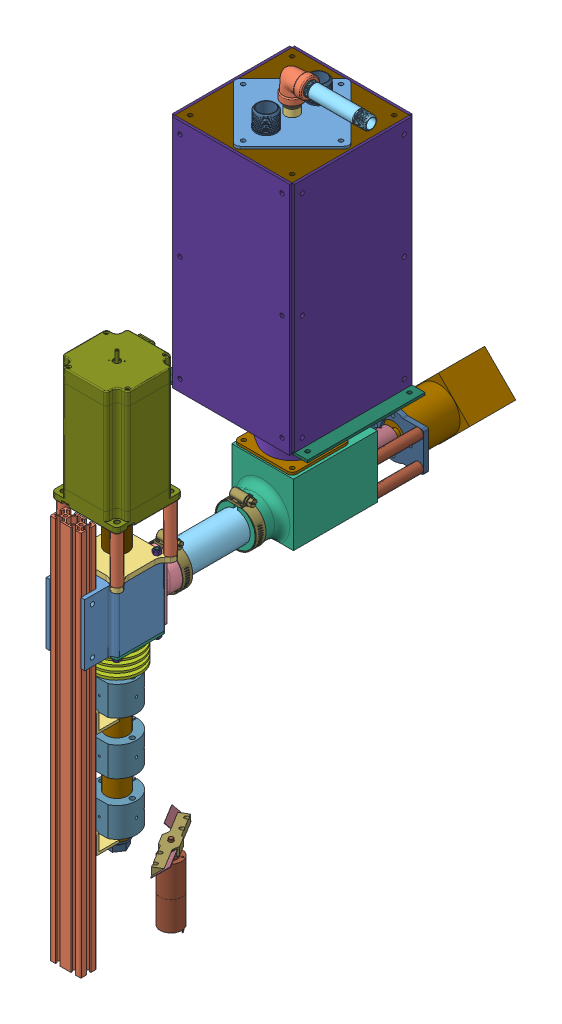
SolidWorks assembly final assembly, configuration Default. Lengths in mm.
Overall size (209.74 884.29 599.56).
88 component instances, 46 part files, 1 mates.
Components (placement in the parent):
- standalone extruder-1: standalone extruder [Default] at (308.2662 326.3295 645.2175) size (88.08 678.87 599.56)
  - hopper rev02-1: hopper rev02 [Default] at (27.6432 17.1739 46.7145) size (63.5 80 98.5)
  - 500mm 2040-1: 500mm 2040 [Default] at (27.6432 169.1296 103.4645) x (0 0 1) z (0 1 0) size (20 40 500)
  - thrust bearing plate-1: thrust bearing plate [Default] at (27.6432 97.1739 46.7145) size (83.7 6.35 85.2)
  - 5909K310_THRUST NEEDLE-ROLLER BEARING-1: 5909K310_THRUST NEEDLE-ROLLER BEARING [5909K31] at (27.6432 95.3689 46.7145) size (23.81 19.84 23.81)
  - 5909K440_THRUST NEEDLE-ROLLER BEARING-1: 5909K440_THRUST NEEDLE-ROLLER BEARING [5909K44] at (27.6432 93.5639 46.7145) x (0 1 0) z (0.735724 0 0.677282) size (0.81 23.81 23.81)
  - 5909K440_THRUST NEEDLE-ROLLER BEARING-2: 5909K440_THRUST NEEDLE-ROLLER BEARING [5909K44] at (27.6432 96.3611 46.7145) x (0 1 0) z (-0.546944 0 0.837169) size (0.81 23.81 23.81)
  - barrel lock mount-1: barrel lock mount [Default] at (27.6432 17.1739 46.7145) x (-1 0 0) z (0 0 1) size (63.5 3.17 63.5)
  - barrel lock-1: barrel lock [Default] at (27.6432 -17.7511 46.7145) x (-0.997738 0 -0.067218) z (0.067218 0 -0.997738) size (60.96 31.75 60.96)
  - screw standin-1: screw standin [Default] at (27.6432 -173.1361 46.7145) x (0.133635 0 0.991031) z (-0.991031 0 0.133635) size (19.05 324.71 19.05)
  - extruder barrel_rev01-1: extruder barrel_rev01 [Default] at (27.6432 93.3739 46.7145) x (1 0 0) z (0 -1 0) size (28.57 28.57 304.8)
  - nozzle_rev01-1: nozzle_rev01 [Default] at (27.6432 -192.3761 46.7145) x (0.565776 0 -0.824559) z (0 -1 0) size (28.57 28.57 31.75)
  - 3262_1-1: 3262_1 [Default] at (38.4207 -337.9043 -12.6632) x (0.853325 0 -0.52138) z (0 1 0) size (28 28 106.2)
  - blade wheel-1: blade wheel [Default] at (38.4207 -243.7043 -12.6632) x (-0.52138 0 -0.853325) z (-0.853325 0 0.52138) size (90 10 20)
  - blade fin-1: blade fin [Default] at (57.514 -246.4382 14.8704) x (-0.653685 -0.642788 0.3994) z (-0.52138 0 -0.853325) size (23.8 0.5 30)
  - blade fin-2: blade fin [Default] at (19.3274 -246.4382 -40.1969) x (0.653685 -0.642788 -0.3994) z (0.52138 0 0.853325) size (23.8 0.5 30)
  - dual cartridge heater block pelletizer-1: dual cartridge heater block pelletizer [Default] at (27.6432 -200.2361 46.7145) x (0 0 1) z (-1 0 0) size (48.25 38.1 50.8)
  - dual cartridge heater block pelletizer-2: dual cartridge heater block pelletizer [Default] at (27.6432 -132.1361 46.7145) x (0 0 1) z (-1 0 0) size (48.25 38.1 50.8)
  - dual cartridge heater block pelletizer-3: dual cartridge heater block pelletizer [Default] at (27.6432 -64.0361 46.7145) x (0 0 1) z (-1 0 0) size (48.25 38.1 50.8)
  - 93325A413_GRADE B7 MEDIUM STRENGTH STEEL THREADED ROD-1: 93325A413_GRADE B7 MEDIUM STRENGTH STEEL THREADED ROD [93325A413] at (53.686 58.9989 20.6718) x (0 -1 0) z (0 0 1) size (101.5 5.07 5.77)
  - 93325A413_GRADE B7 MEDIUM STRENGTH STEEL THREADED ROD-2: 93325A413_GRADE B7 MEDIUM STRENGTH STEEL THREADED ROD [93325A413] at (53.686 58.9989 72.7573) x (0 -1 0) z (-0.546944 0 0.837169) size (101.5 5.07 5.77)
  - 93325A413_GRADE B7 MEDIUM STRENGTH STEEL THREADED ROD-3: 93325A413_GRADE B7 MEDIUM STRENGTH STEEL THREADED ROD [93325A413] at (1.6005 58.9989 72.7573) x (0 1 0) z (-0.546944 0 0.837169) size (101.5 5.07 5.77)
  - 93325A413_GRADE B7 MEDIUM STRENGTH STEEL THREADED ROD-4: 93325A413_GRADE B7 MEDIUM STRENGTH STEEL THREADED ROD [93325A413] at (1.6005 58.9989 20.6718) x (0 -1 0) z (-0.546944 0 0.837169) size (101.5 5.07 5.77)
  - nema 34-1: nema 34 [Default] at (27.6432 165.5239 46.7145) x (1 0 0) z (0 -1 0) size (85.21 93.2 198.32)
  - 94645A102_ZINC-PLATED CLASS 10 STL NYLON-INSERT LOCKNUT-1: 94645A102_ZINC-PLATED CLASS 10 STL NYLON-INSERT LOCKNUT [94645A102] at (53.686 103.5239 72.7573) size (8 5.15 9.24)
  - 94645A102_ZINC-PLATED CLASS 10 STL NYLON-INSERT LOCKNUT-2: 94645A102_ZINC-PLATED CLASS 10 STL NYLON-INSERT LOCKNUT [94645A102] at (53.686 103.5239 20.6718) size (8 5.15 9.24)
  - 94645A102_ZINC-PLATED CLASS 10 STL NYLON-INSERT LOCKNUT-3: 94645A102_ZINC-PLATED CLASS 10 STL NYLON-INSERT LOCKNUT [94645A102] at (1.6005 103.5239 72.7573) size (8 5.15 9.24)
  - 94645A102_ZINC-PLATED CLASS 10 STL NYLON-INSERT LOCKNUT-4: 94645A102_ZINC-PLATED CLASS 10 STL NYLON-INSERT LOCKNUT [94645A102] at (1.6005 103.5239 20.6718) size (8 5.15 9.24)
  - 94645A102_ZINC-PLATED CLASS 10 STL NYLON-INSERT LOCKNUT-5: 94645A102_ZINC-PLATED CLASS 10 STL NYLON-INSERT LOCKNUT [94645A102] at (53.686 13.9989 20.6718) x (-0.5 0 -0.866025) z (-0.866025 0 0.5) size (8 5.15 9.24)
  - 94645A102_ZINC-PLATED CLASS 10 STL NYLON-INSERT LOCKNUT-6: 94645A102_ZINC-PLATED CLASS 10 STL NYLON-INSERT LOCKNUT [94645A102] at (53.686 13.9989 72.7573) x (-0.5 0 -0.866025) z (-0.866025 0 0.5) size (8 5.15 9.24)
  - 94645A102_ZINC-PLATED CLASS 10 STL NYLON-INSERT LOCKNUT-7: 94645A102_ZINC-PLATED CLASS 10 STL NYLON-INSERT LOCKNUT [94645A102] at (1.6005 13.9989 72.7573) x (-0.5 0 -0.866025) z (-0.866025 0 0.5) size (8 5.15 9.24)
  - 94645A102_ZINC-PLATED CLASS 10 STL NYLON-INSERT LOCKNUT-8: 94645A102_ZINC-PLATED CLASS 10 STL NYLON-INSERT LOCKNUT [94645A102] at (1.6005 13.9989 20.6718) x (-0.5 0 -0.866025) z (-0.866025 0 0.5) size (8 5.15 9.24)
  - motor coupler-1: motor coupler [Default] at (27.6432 111.6639 46.7145) x (-1 0 0) z (0 0 -1) size (28.57 40 28.57)
  - 93245A110_NONMARRING FLAT POINT SOCKET SET SCREW-3: 93245A110_NONMARRING FLAT POINT SOCKET SET SCREW [93245A110] at (27.6432 145.3139 34.7745) x (-0.923728 -0.383049 0) z (0 0 -1) size (4.62 4.16 4.74)
  - 93245A110_NONMARRING FLAT POINT SOCKET SET SCREW-4: 93245A110_NONMARRING FLAT POINT SOCKET SET SCREW [93245A110] at (19.2932 118.0139 46.7145) x (0 0.992337 0.12356) z (-1 0 0) size (4.62 4.16 4.74)
  - 93245A110_NONMARRING FLAT POINT SOCKET SET SCREW-5: 93245A110_NONMARRING FLAT POINT SOCKET SET SCREW [93245A110] at (27.6432 118.0139 38.3645) x (-0.923728 -0.383049 0) z (0 0 -1) size (4.62 4.16 4.74)
  - 93245A110_NONMARRING FLAT POINT SOCKET SET SCREW-6: 93245A110_NONMARRING FLAT POINT SOCKET SET SCREW [93245A110] at (17.7057 145.3139 46.7145) x (0 0.989125 0.14708) z (-1 0 0) size (4.62 4.16 4.74)
  - 93245A110_NONMARRING FLAT POINT SOCKET SET SCREW-8: 93245A110_NONMARRING FLAT POINT SOCKET SET SCREW [93245A110] at (29.1991 1.5816 32.0423) x (-0.924173 -0.376865 -0.062262) z (0.067218 0 -0.997738) size (4.62 4.16 4.74)
  - motor standoff-1: motor standoff [Default] at (62.3932 103.5239 81.4645) size (12.7 62 12.7)
  - motor standoff-2: motor standoff [Default] at (62.3932 103.5239 11.9645) size (12.7 62 12.7)
  - motor standoff-3: motor standoff [Default] at (-7.1068 103.5239 81.4645) size (12.7 62 12.7)
  - motor standoff-4: motor standoff [Default] at (-7.1068 103.5239 11.9645) size (12.7 62 12.7)
  - extruder support-1: extruder support [Default] at (7.6432 -203.4111 93.4645) x (0 -1 0) z (0 0 1) size (25.4 40 31.75)
  - extruder support-2: extruder support [Default] at (7.6432 -67.2111 93.4645) x (0 -1 0) z (0 0 1) size (25.4 40 31.75)
  - auger feed-1: auger feed [Default] at (27.6432 57.1739 9.9645) size (57.15 80 40)
  - agure feed tube-1: agure feed tube [Default] at (27.6432 57.1739 -142.4355) x (0.920148 -0.391572 0) z (0 0 1) size (38.1 38.1 152.4)
  - dryer to feeder hopper-1: dryer to feeder hopper [Default] at (27.6432 57.1739 -142.4355) x (-1 0 0) z (0 0 -1) size (80 80.4 143.9)
  - feed screw-1: feed screw [Default] at (27.6432 57.1739 168.8745) x (0.990824 -0.135162 0) z (0 0 -1) size (32.68 31.75 457.2)
  - 60355K601_BALL BEARING-1: 60355K601_BALL BEARING [60355K601] at (27.6432 56.5563 -245.3042) size (28.57 28.57 7.94)
  - motor planetary standin nema 23-1: motor planetary standin nema 23 [Default] at (27.6432 57.1739 -370.6855) x (0.707107 -0.707107 0) z (-0.707107 -0.707107 0) size (57 141 57)
  - motor mount nema 23-1: motor mount nema 23 [Default] at (27.6432 57.1739 -311.3355) x (1 0 0) z (0 1 0) size (80 6.35 57)
  - nema 23 standoff-1: nema 23 standoff [Default] at (61.2932 76.2239 -311.3355) size (12.7 12.7 60)
  - nema 23 standoff-2: nema 23 standoff [Default] at (-6.0068 76.2239 -311.3355) size (12.7 12.7 60)
  - nema 23 standoff-3: nema 23 standoff [Default] at (61.2932 38.1239 -311.3355) size (12.7 12.7 60)
  - nema 23 standoff-4: nema 23 standoff [Default] at (-6.0068 38.1239 -311.3355) size (12.7 12.7 60)
  - 5415K180_WORM-DRIVE CLAMPS FOR FIRM HOSE AND TUBE-1: 5415K180_WORM-DRIVE CLAMPS FOR FIRM HOSE AND TUBE [5415K18] at (27.6432 57.1739 -113.7855) size (53.24 62.22 17.02)
  - 5415K180_WORM-DRIVE CLAMPS FOR FIRM HOSE AND TUBE-2: 5415K180_WORM-DRIVE CLAMPS FOR FIRM HOSE AND TUBE [5415K18] at (27.6432 57.1739 -18.6855) size (53.24 62.22 17.02)
  - nema 23 coupler-1: nema 23 coupler [Default] at (27.6432 57.1739 -269.9105) x (-0.925659 -0.378358 0) z (0.378358 -0.925659 0) size (25.4 36.83 25.4)
- dryer stand alone-1: dryer stand alone [Default] at (232.5423 442.5987 278.9982) size (209.74 423.31 158.7)
  - tube-1: tube [Default] at (103.5422 61.3012 185.6839) size (164.34 304.8 101.6)
  - flange rev01-1: flange rev01 [Default] at (103.5422 61.3012 185.6839) x (-1 0 0) z (0 0 -1) size (192.4 3.17 152.4)
  - HFS5-2020-299-1: HFS5-2020-299 [Default] at (169.7422 63.9262 119.4839) x (-1 0 0) z (0 -1 0) size (20 20 298.45)
  - HFS5-2020-299-2: HFS5-2020-299 [Default] at (37.3422 63.9262 119.4839) x (-1 0 0) z (0 -1 0) size (20 20 298.45)
  - HFS5-2020-299-3: HFS5-2020-299 [Default] at (169.7422 63.9262 251.8839) x (-1 0 0) z (0 -1 0) size (20 20 298.45)
  - HFS5-2020-299-4: HFS5-2020-299 [Default] at (37.3422 363.4762 251.8839) x (-1 0 0) z (0 1 0) size (20 20 298.45)
  - side plate 1_16-1: side plate 1_16 [Default] at (103.5422 213.7012 263.4587) x (-1 0 0) z (0 0 -1) size (152.4 304.8 1.57)
  - side plate 1_16-2: side plate 1_16 [Default] at (103.5422 213.7012 265.0335) x (-1 0 0) z (0 0 -1) size (152.4 304.8 1.57)
  - flange rev02-1: flange rev02 [Default] at (103.5422 362.9262 185.6839) x (-1 0 0) z (0 0 -1) size (152.4 3.17 152.4)
  - top cover-1: top cover [Default] at (103.5422 369.2762 185.6839) x (-0.707107 0 -0.707107) z (0 -1 0) size (107.76 107.76 3.17)
  - 4452K413_TYPE 316 STAINLESS STL THREADED PIPE FITTING-2: 4452K413_TYPE 316 STAINLESS STL THREADED PIPE FITTING [4452K413] at (103.5422 407.8982 185.6839) x (-1 0 0) z (0 0 1) size (37.28 37.03 30.11)
  - 4548K159_STD-WALL TYPE 316-316L SS THRD PIPE NIPPLE-1: 4548K159_STD-WALL TYPE 316-316L SS THRD PIPE NIPPLE [4548K159] at (103.5422 292.6762 185.6839) x (0 1 0) z (0 0 1) size (203.35 17.91 17.78)
  - 4464K498_TYPE 304 STAINLESS STL THREADED PIPE FITTING-1: 4464K498_TYPE 304 STAINLESS STL THREADED PIPE FITTING [4464K498] at (103.5422 180.2482 185.6839) x (-0.837169 0 -0.546944) z (0 1 0) size (25.91 25.91 21.03)
  - 4548K145_STD-WALL TYPE 316-316L SS THRD PIPE NIPPLE-2: 4548K145_STD-WALL TYPE 316-316L SS THRD PIPE NIPPLE [4548K145] at (161.6142 407.8982 185.6839) x (1 0 0) z (0 -0.851872 -0.523749) size (89.04 17.99 18.06)
  - heater band-1: heater band [Default] at (103.5422 257.8762 185.6839) size (116.47 50.8 107.95)
  - heater band-2: heater band [Default] at (103.5422 132.2762 185.6839) size (116.47 50.8 107.95)
  - heater band-3: heater band [Default] at (103.5422 69.4762 185.6839) size (116.47 50.8 107.95)
  - heater band-4: heater band [Default] at (103.5422 195.0762 185.6839) size (116.47 50.8 107.95)
  - bottom cover-1: bottom cover [Default] at (103.6306 61.3012 185.6839) x (-0.707107 0 -0.707107) z (0 -1 0) size (107.76 107.76 3.17)
  - nozzle reduction-1: nozzle reduction [Default] at (103.6306 61.3012 185.6839) x (-0.837169 0 -0.546944) z (-0.546944 0 0.837169) size (101.6 63.5 101.6)
  - 2.5 in bracket-1: 2.5 in bracket [Default] at (103.6306 -2.1988 185.6839) size (76.2 3.17 76.2)
  - side plate 1_16-7: side plate 1_16 [Default] at (103.5422 213.7012 107.9091) size (152.4 304.8 1.57)
  - side plate 1_16-8: side plate 1_16 [Default] at (103.5422 213.7012 106.3343) size (152.4 304.8 1.57)
  - 9157K150_STD-WALL 304-304L SS THRD ONE END PIPE NIPPLE-1: 9157K150_STD-WALL 304-304L SS THRD ONE END PIPE NIPPLE [9157K15] at (103.5422 378.8012 152.0289) x (0 1 0) z (-0.332767 0 0.943009) size (25.49 27.89 27.84)
  - 9157K150_STD-WALL 304-304L SS THRD ONE END PIPE NIPPLE-2: 9157K150_STD-WALL 304-304L SS THRD ONE END PIPE NIPPLE [9157K15] at (103.5422 378.8012 219.3389) x (0 1 0) z (-0.546944 0 0.837169) size (25.49 27.89 27.84)
  - side plate 1_16-9: side plate 1_16 [Default] at (182.8918 213.7012 185.6839) x (0 0 1) z (-1 0 0) size (152.4 304.8 1.57)
  - side plate 1_16-10: side plate 1_16 [Default] at (181.317 213.7012 185.6839) x (0 0 1) z (-1 0 0) size (152.4 304.8 1.57)
  - side plate 1_16-11: side plate 1_16 [Default] at (27.3422 213.7012 185.6839) x (0 0 1) z (-1 0 0) size (152.4 304.8 1.57)
  - side plate 1_16-12: side plate 1_16 [Default] at (25.7674 213.7012 185.6839) x (0 0 1) z (-1 0 0) size (152.4 304.8 1.57)
Mates (geometry in assembly coordinates):
- Coincident1: coincident aligned: plane of standalone extruder-1/dryer to feeder hopper-1 through (335.9095 383.5035 502.7821) normal (0 0 1); plane of dryer stand alone-1/2.5 in bracket-1 through (298.0729 443.5749 502.7821) normal (0 0 1)
